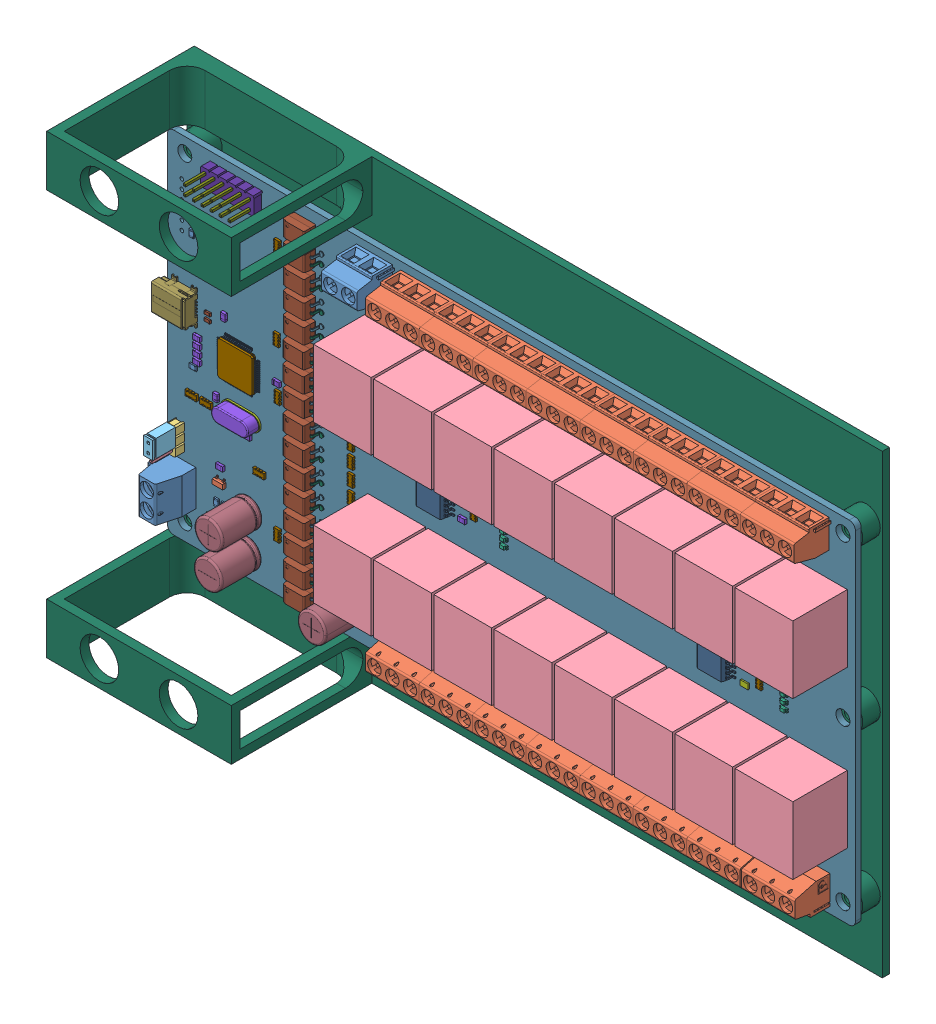
SolidWorks assembly Assem2, configuration Default. Lengths in mm. (continued)
Components (placement in the parent): (continued)
- 16_Channel_USB_Relay.step-1: 16_Channel_USB_Relay.step [Default] at (-11.9082 58.988 141.1455) size (200.04 103.47 20) (continued)
  - U12.step-1: U12.step [Default] at origin size (10 4.58 3.85) (continued)
    - User_Library-PC817_Gullwing.step-1: User_Library-PC817_Gullwing.step [Default] at (39.6975 47.1295 2.1) x (0 -1 0) z (-1 0 0) size (4.58 3.85 10) (continued)
      - User_Library-PC817_Gullwing_Gullwing_Pin_MIR_MIR.step-1: User_Library-PC817_Gullwing_Gullwing_Pin_MIR_MIR.step [Default] at (13.5652 -2.1015 0.2722) x (-1 0 0) z (0 0 -1) size (1.2 2.23 1.87)
  - U11.step-1: U11.step [Default] at origin size (10 4.58 3.85)
    - User_Library-PC817_Gullwing.step-1: User_Library-PC817_Gullwing.step [Default] at (39.6213 53.2509 2.1) x (0 -1 0) z (-1 0 0) size (4.58 3.85 10)
      - User_Library-PC817_Gullwing_PC817_Body.step-1: User_Library-PC817_Gullwing_PC817_Body.step [Default] at origin size (4.58 3.5 6.5)
      - User_Library-PC817_Gullwing_Gullwing_Pin.step-1: User_Library-PC817_Gullwing_Gullwing_Pin.step [Default] at (-13.5652 -2.1015 -0.2722) size (1.2 2.23 1.87)
      - User_Library-PC817_Gullwing_Gullwing_Pin_MIR.step-1: User_Library-PC817_Gullwing_Gullwing_Pin_MIR.step [Default] at (13.5652 -2.1015 -0.2722) x (-1 0 0) z (0 0 -1) size (1.2 2.23 1.87)
      - User_Library-PC817_Gullwing_Gullwing_Pin_MIR1.step-1: User_Library-PC817_Gullwing_Gullwing_Pin_MIR1.step [Default] at (-13.5652 -2.1015 0.2722) size (1.2 2.23 1.87)
      - User_Library-PC817_Gullwing_Gullwing_Pin_MIR_MIR.step-1: User_Library-PC817_Gullwing_Gullwing_Pin_MIR_MIR.step [Default] at (13.5652 -2.1015 0.2722) x (-1 0 0) z (0 0 -1) size (1.2 2.23 1.87)
  - U10.step-1: U10.step [Default] at origin size (10 4.58 3.85)
    - User_Library-PC817_Gullwing.step-1: User_Library-PC817_Gullwing.step [Default] at (39.6213 59.2199 2.1) x (0 -1 0) z (-1 0 0) size (4.58 3.85 10)
      - User_Library-PC817_Gullwing_PC817_Body.step-1: User_Library-PC817_Gullwing_PC817_Body.step [Default] at origin size (4.58 3.5 6.5)
      - User_Library-PC817_Gullwing_Gullwing_Pin.step-1: User_Library-PC817_Gullwing_Gullwing_Pin.step [Default] at (-13.5652 -2.1015 -0.2722) size (1.2 2.23 1.87)
      - User_Library-PC817_Gullwing_Gullwing_Pin_MIR.step-1: User_Library-PC817_Gullwing_Gullwing_Pin_MIR.step [Default] at (13.5652 -2.1015 -0.2722) x (-1 0 0) z (0 0 -1) size (1.2 2.23 1.87)
      - User_Library-PC817_Gullwing_Gullwing_Pin_MIR1.step-1: User_Library-PC817_Gullwing_Gullwing_Pin_MIR1.step [Default] at (-13.5652 -2.1015 0.2722) size (1.2 2.23 1.87)
      - User_Library-PC817_Gullwing_Gullwing_Pin_MIR_MIR.step-1: User_Library-PC817_Gullwing_Gullwing_Pin_MIR_MIR.step [Default] at (13.5652 -2.1015 0.2722) x (-1 0 0) z (0 0 -1) size (1.2 2.23 1.87)
  - U9.step-1: U9.step [Default] at origin size (10 4.58 3.85)
    - User_Library-PC817_Gullwing.step-1: User_Library-PC817_Gullwing.step [Default] at (39.6975 65.2651 2.1) x (0 -1 0) z (-1 0 0) size (4.58 3.85 10)
      - User_Library-PC817_Gullwing_PC817_Body.step-1: User_Library-PC817_Gullwing_PC817_Body.step [Default] at origin size (4.58 3.5 6.5)
      - User_Library-PC817_Gullwing_Gullwing_Pin.step-1: User_Library-PC817_Gullwing_Gullwing_Pin.step [Default] at (-13.5652 -2.1015 -0.2722) size (1.2 2.23 1.87)
      - User_Library-PC817_Gullwing_Gullwing_Pin_MIR.step-1: User_Library-PC817_Gullwing_Gullwing_Pin_MIR.step [Default] at (13.5652 -2.1015 -0.2722) x (-1 0 0) z (0 0 -1) size (1.2 2.23 1.87)
      - User_Library-PC817_Gullwing_Gullwing_Pin_MIR1.step-1: User_Library-PC817_Gullwing_Gullwing_Pin_MIR1.step [Default] at (-13.5652 -2.1015 0.2722) size (1.2 2.23 1.87)
      - User_Library-PC817_Gullwing_Gullwing_Pin_MIR_MIR.step-1: User_Library-PC817_Gullwing_Gullwing_Pin_MIR_MIR.step [Default] at (13.5652 -2.1015 0.2722) x (-1 0 0) z (0 0 -1) size (1.2 2.23 1.87)
  - U8.step-1: U8.step [Default] at origin size (10 4.58 3.85)
    - User_Library-PC817_Gullwing.step-1: User_Library-PC817_Gullwing.step [Default] at (39.7229 71.3865 2.1) x (0 -1 0) z (-1 0 0) size (4.58 3.85 10)
      - User_Library-PC817_Gullwing_PC817_Body.step-1: User_Library-PC817_Gullwing_PC817_Body.step [Default] at origin size (4.58 3.5 6.5)
      - User_Library-PC817_Gullwing_Gullwing_Pin.step-1: User_Library-PC817_Gullwing_Gullwing_Pin.step [Default] at (-13.5652 -2.1015 -0.2722) size (1.2 2.23 1.87)
      - User_Library-PC817_Gullwing_Gullwing_Pin_MIR.step-1: User_Library-PC817_Gullwing_Gullwing_Pin_MIR.step [Default] at (13.5652 -2.1015 -0.2722) x (-1 0 0) z (0 0 -1) size (1.2 2.23 1.87)
      - User_Library-PC817_Gullwing_Gullwing_Pin_MIR1.step-1: User_Library-PC817_Gullwing_Gullwing_Pin_MIR1.step [Default] at (-13.5652 -2.1015 0.2722) size (1.2 2.23 1.87)
      - User_Library-PC817_Gullwing_Gullwing_Pin_MIR_MIR.step-1: User_Library-PC817_Gullwing_Gullwing_Pin_MIR_MIR.step [Default] at (13.5652 -2.1015 0.2722) x (-1 0 0) z (0 0 -1) size (1.2 2.23 1.87)
  - U7.step-1: U7.step [Default] at origin size (10 4.58 3.85)
    - User_Library-PC817_Gullwing.step-1: User_Library-PC817_Gullwing.step [Default] at (39.7737 77.4317 2.1) x (0 -1 0) z (-1 0 0) size (4.58 3.85 10)
      - User_Library-PC817_Gullwing_PC817_Body.step-1: User_Library-PC817_Gullwing_PC817_Body.step [Default] at origin size (4.58 3.5 6.5)
      - User_Library-PC817_Gullwing_Gullwing_Pin.step-1: User_Library-PC817_Gullwing_Gullwing_Pin.step [Default] at (-13.5652 -2.1015 -0.2722) size (1.2 2.23 1.87)
      - User_Library-PC817_Gullwing_Gullwing_Pin_MIR.step-1: User_Library-PC817_Gullwing_Gullwing_Pin_MIR.step [Default] at (13.5652 -2.1015 -0.2722) x (-1 0 0) z (0 0 -1) size (1.2 2.23 1.87)
      - User_Library-PC817_Gullwing_Gullwing_Pin_MIR1.step-1: User_Library-PC817_Gullwing_Gullwing_Pin_MIR1.step [Default] at (-13.5652 -2.1015 0.2722) size (1.2 2.23 1.87)
      - User_Library-PC817_Gullwing_Gullwing_Pin_MIR_MIR.step-1: User_Library-PC817_Gullwing_Gullwing_Pin_MIR_MIR.step [Default] at (13.5652 -2.1015 0.2722) x (-1 0 0) z (0 0 -1) size (1.2 2.23 1.87)
  - U6.step-1: U6.step [Default] at origin size (10 4.58 3.85)
    - User_Library-PC817_Gullwing.step-1: User_Library-PC817_Gullwing.step [Default] at (39.7737 83.2991 2.1) x (0 -1 0) z (-1 0 0) size (4.58 3.85 10)
      - User_Library-PC817_Gullwing_PC817_Body.step-1: User_Library-PC817_Gullwing_PC817_Body.step [Default] at origin size (4.58 3.5 6.5)
      - User_Library-PC817_Gullwing_Gullwing_Pin.step-1: User_Library-PC817_Gullwing_Gullwing_Pin.step [Default] at (-13.5652 -2.1015 -0.2722) size (1.2 2.23 1.87)
      - User_Library-PC817_Gullwing_Gullwing_Pin_MIR.step-1: User_Library-PC817_Gullwing_Gullwing_Pin_MIR.step [Default] at (13.5652 -2.1015 -0.2722) x (-1 0 0) z (0 0 -1) size (1.2 2.23 1.87)
      - User_Library-PC817_Gullwing_Gullwing_Pin_MIR1.step-1: User_Library-PC817_Gullwing_Gullwing_Pin_MIR1.step [Default] at (-13.5652 -2.1015 0.2722) size (1.2 2.23 1.87)
      - User_Library-PC817_Gullwing_Gullwing_Pin_MIR_MIR.step-1: User_Library-PC817_Gullwing_Gullwing_Pin_MIR_MIR.step [Default] at (13.5652 -2.1015 0.2722) x (-1 0 0) z (0 0 -1) size (1.2 2.23 1.87)
  - U5.step-1: U5.step [Default] at origin size (10 4.58 3.85)
    - User_Library-PC817_Gullwing.step-1: User_Library-PC817_Gullwing.step [Default] at (39.7737 89.2681 2.1) x (0 -1 0) z (-1 0 0) size (4.58 3.85 10)
      - User_Library-PC817_Gullwing_PC817_Body.step-1: User_Library-PC817_Gullwing_PC817_Body.step [Default] at origin size (4.58 3.5 6.5)
      - User_Library-PC817_Gullwing_Gullwing_Pin.step-1: User_Library-PC817_Gullwing_Gullwing_Pin.step [Default] at (-13.5652 -2.1015 -0.2722) size (1.2 2.23 1.87)
      - User_Library-PC817_Gullwing_Gullwing_Pin_MIR.step-1: User_Library-PC817_Gullwing_Gullwing_Pin_MIR.step [Default] at (13.5652 -2.1015 -0.2722) x (-1 0 0) z (0 0 -1) size (1.2 2.23 1.87)
      - User_Library-PC817_Gullwing_Gullwing_Pin_MIR1.step-1: User_Library-PC817_Gullwing_Gullwing_Pin_MIR1.step [Default] at (-13.5652 -2.1015 0.2722) size (1.2 2.23 1.87)
      - User_Library-PC817_Gullwing_Gullwing_Pin_MIR_MIR.step-1: User_Library-PC817_Gullwing_Gullwing_Pin_MIR_MIR.step [Default] at (13.5652 -2.1015 0.2722) x (-1 0 0) z (0 0 -1) size (1.2 2.23 1.87)
  - U4.step-1: U4.step [Default] at origin size (10 4.58 3.85)
    - User_Library-PC817_Gullwing.step-1: User_Library-PC817_Gullwing.step [Default] at (39.7737 95.1355 2.1) x (0 -1 0) z (-1 0 0) size (4.58 3.85 10)
      - User_Library-PC817_Gullwing_PC817_Body.step-1: User_Library-PC817_Gullwing_PC817_Body.step [Default] at origin size (4.58 3.5 6.5)
      - User_Library-PC817_Gullwing_Gullwing_Pin.step-1: User_Library-PC817_Gullwing_Gullwing_Pin.step [Default] at (-13.5652 -2.1015 -0.2722) size (1.2 2.23 1.87)
      - User_Library-PC817_Gullwing_Gullwing_Pin_MIR.step-1: User_Library-PC817_Gullwing_Gullwing_Pin_MIR.step [Default] at (13.5652 -2.1015 -0.2722) x (-1 0 0) z (0 0 -1) size (1.2 2.23 1.87)
      - User_Library-PC817_Gullwing_Gullwing_Pin_MIR1.step-1: User_Library-PC817_Gullwing_Gullwing_Pin_MIR1.step [Default] at (-13.5652 -2.1015 0.2722) size (1.2 2.23 1.87)
      - User_Library-PC817_Gullwing_Gullwing_Pin_MIR_MIR.step-1: User_Library-PC817_Gullwing_Gullwing_Pin_MIR_MIR.step [Default] at (13.5652 -2.1015 0.2722) x (-1 0 0) z (0 0 -1) size (1.2 2.23 1.87)
  - P1.step-1: P1.step [Default] at origin size (15.24 5.08 11.54)
    - STEP-61301221121-rev1.step-1: STEP-61301221121-rev1.step [Default] at (19.7712 96.3422 1.3) x (-1 0 0) z (0 1 0) size (15.24 11.54 5.08)
      - 6130xx21121_PIN.step-1: 6130xx21121_PIN.step [Default] at (-6.35 1.5 0) x (1 0 0) z (0 -1 0) size (0.64 0.64 11.54)
      - 6130xx21121_PIN.step-2: 6130xx21121_PIN.step [Default] at (-6.35 1.5 -2.54) x (1 0 0) z (0 -1 0) size (0.64 0.64 11.54)
      - 6130xx21121_PIN.step-3: 6130xx21121_PIN.step [Default] at (-3.81 1.5 0) x (1 0 0) z (0 -1 0) size (0.64 0.64 11.54)
      - 6130xx21121_PIN.step-4: 6130xx21121_PIN.step [Default] at (-3.81 1.5 -2.54) x (1 0 0) z (0 -1 0) size (0.64 0.64 11.54)
      - 6130xx21121_PIN.step-5: 6130xx21121_PIN.step [Default] at (-1.27 1.5 0) x (1 0 0) z (0 -1 0) size (0.64 0.64 11.54)
      - 6130xx21121_PIN.step-6: 6130xx21121_PIN.step [Default] at (-1.27 1.5 -2.54) x (1 0 0) z (0 -1 0) size (0.64 0.64 11.54)
      - 6130xx21121_PIN.step-7: 6130xx21121_PIN.step [Default] at (1.27 1.5 0) x (1 0 0) z (0 -1 0) size (0.64 0.64 11.54)
      - 6130xx21121_PIN.step-8: 6130xx21121_PIN.step [Default] at (1.27 1.5 -2.54) x (1 0 0) z (0 -1 0) size (0.64 0.64 11.54)
      - 6130xx21121_PIN.step-9: 6130xx21121_PIN.step [Default] at (3.81 1.5 0) x (1 0 0) z (0 -1 0) size (0.64 0.64 11.54)
      - 6130xx21121_PIN.step-10: 6130xx21121_PIN.step [Default] at (3.81 1.5 -2.54) x (1 0 0) z (0 -1 0) size (0.64 0.64 11.54)
      - 6130xx21121_PIN.step-11: 6130xx21121_PIN.step [Default] at (6.35 1.5 0) x (1 0 0) z (0 -1 0) size (0.64 0.64 11.54)
      - 6130xx21121_PIN.step-12: 6130xx21121_PIN.step [Default] at (6.35 1.5 -2.54) x (1 0 0) z (0 -1 0) size (0.64 0.64 11.54)
      - 61301221121.step-1: 61301221121.step [Default] at origin size (15.24 2.54 5.08)
  - P5.step-1: P5.step [Default] at origin size (8.1 10.73 13.5)
    - 1729128_07.step-1: 1729128_07.step [Default] at (0.7762 20.5414 0) x (-1 0 0) z (0 1 0) size (8.1 13.5 10.73)
      - mkdsn_1.5-2-5.08.step-1: mkdsn_1.5-2-5.08.step [Default] at (-39.331 -15.5089 -8.19) x (-1 0 0) z (0 0 -1) size (8.1 13.5 10.73)
  - U2.step-1: U2.step [Default] at origin size (8.15 10.72 7.75)
    - SOT-223.step-1: SOT-223.step [Default] at (14.0941 7.1499 0) x (-1 0 0) z (0 0 1) size (8.15 10.72 7.75)
  - R13.step-1: R13.step [Default] at origin size (1.6 3.2 0.65)
    - User_Library-resnet.step-1: User_Library-resnet.step [Default] at (31.7979 15.3035 0) x (0 1 0) z (1 0 0) size (3.2 0.65 1.6)
  - R3.step-1: R3.step [Default] at origin size (1.25 2 0.47)
    - SW3dPS-R0805.step-1: SW3dPS-R0805.step [Default] at (16.4057 14.5159 -0.05) x (0 -1 0) z (0 0 1) size (2 1.25 0.47)
  - R4.step-1: R4.step [Default] at origin size (1.25 2 0.47)
    - SW3dPS-R0805.step-1: SW3dPS-R0805.step [Default] at (14.3991 14.5159 -0.05) x (0 -1 0) z (0 0 1) size (2 1.25 0.47)
  - D1.step-1: D1.step [Default] at origin size (3 2.5 1.1)
    - CircuitWorks-SOT-23.step-1: CircuitWorks-SOT-23.step [Default] at (15.4911 19.9515 0.5541) x (1 0 0) z (0 -1 0) size (3 1.1 2.5)
  - C12.step-1: C12.step [Default] at origin size (2 1.31 0.76)
    - SW3DPS-CAPACITOR_0805-DEFAULT.step-1: SW3DPS-CAPACITOR_0805-DEFAULT.step [Default] at (15.5419 23.9139 0) x (1 0 0) z (0 -1 0) size (2 0.76 1.31)
  - K1.step-1: K1.step [Default] at origin size (2.61 7.64 12.07)
    - jmper.step-1: jmper.step [Default] at (3.7564 25.7682 1.25) x (-0.008727 0.999962 0) z (0.999962 0.008727 0) size (7.62 11.54 2.54)
      - 61300311121.step-1: 61300311121.step [Default] at origin size (7.62 2.54 2.54)
      - 6130xx11121_PIN.step-1: 6130xx11121_PIN.step [Default] at (-2.54 1.5 0) x (1 0 0) z (0 -1 0) size (0.64 0.64 11.54)
      - 6130xx11121_PIN.step-2: 6130xx11121_PIN.step [Default] at (0 1.5 0) x (1 0 0) z (0 -1 0) size (0.64 0.64 11.54)
      - 6130xx11121_PIN.step-3: 6130xx11121_PIN.step [Default] at (2.54 1.5 0) x (1 0 0) z (0 -1 0) size (0.64 0.64 11.54)
    - pcb_connector_999-19-210-00.step-1: pcb_connector_999-19-210-00.step [Default] at (3.7563 27.0383 2.55) x (0 -1 0) z (-1 0 0) size (5 6.5 2.54)
  - R1.step-1: R1.step [Default] at origin size (3.2 1.6 0.65)
    - User_Library-resnet.step-1: User_Library-resnet.step [Default] at (26.6925 27.9525 0) x (-1 0 0) z (0 1 0) size (3.2 0.65 1.6)
  - C2.step-1: C2.step [Default] at origin size (2 1.31 0.76)
    - SW3DPS-CAPACITOR_0805-DEFAULT.step-1: SW3DPS-CAPACITOR_0805-DEFAULT.step [Default] at (23.3143 35.3947 0) x (1 0 0) z (0 -1 0) size (2 0.76 1.31)
  - C1.step-1: C1.step [Default] at origin size (2 1.31 0.76)
    - SW3DPS-CAPACITOR_0805-DEFAULT.step-1: SW3DPS-CAPACITOR_0805-DEFAULT.step [Default] at (19.7583 35.3947 0) x (1 0 0) z (0 -1 0) size (2 0.76 1.31)
  - X1.step-1: X1.step [Default] at origin size (10.98 4.49 6.6)
    - User_Library-HC49S-1.step-1: User_Library-HC49S-1.step [Default] at (23.8241 39.3469 0) x (-1 0 0) z (0 0 1) size (10.98 4.49 6.6)
      - User_Library-HC49S-1_Fusion.step-1: User_Library-HC49S-1_Fusion.step [Default] at origin size (5.32 0.44 3)
      - User_Library-HC49S-1_Fillet.step-1: User_Library-HC49S-1_Fillet.step [Default] at origin size (10.98 4.49 0.5)
      - User_Library-HC49S-1_Fillet002.step-1: User_Library-HC49S-1_Fillet002.step [Default] at origin size (10.48 3.99 3.5)
  - R7.step-1: R7.step [Default] at origin size (3.2 1.6 0.65)
    - User_Library-resnet.step-1: User_Library-resnet.step [Default] at (11.4957 37.6049 0) x (1 0 0) z (0 -1 0) size (3.2 0.65 1.6)
  - R6.step-1: R6.step [Default] at origin size (3.2 1.6 0.65)
    - User_Library-resnet.step-1: User_Library-resnet.step [Default] at (7.4317 37.5795 0) x (1 0 0) z (0 -1 0) size (3.2 0.65 1.6)
  - C7.step-1: C7.step [Default] at origin size (1.31 2 0.76)
    - SW3DPS-CAPACITOR_0805-DEFAULT.step-1: SW3DPS-CAPACITOR_0805-DEFAULT.step [Default] at (14.3735 40.5765 0) x (0 -1 0) z (-1 0 0) size (2 0.76 1.31)
  - R9.step-1: R9.step [Default] at origin size (2 1.25 0.47)
    - SW3dPS-R0805.step-1: SW3dPS-R0805.step [Default] at (7.7695 44.6149 -0.05) x (-1 0 0) z (0 0 1) size (2 1.25 0.47)
  - C4.step-1: C4.step [Default] at origin size (2 1.31 0.76)
    - SW3DPS-CAPACITOR_0805-DEFAULT.step-1: SW3DPS-CAPACITOR_0805-DEFAULT.step [Default] at (8.9889 46.5709 0) x (-1 0 0) z (0 1 0) size (2 0.76 1.31)
  - C8.step-1: C8.step [Default] at origin size (2 1.31 0.76)
    - SW3DPS-CAPACITOR_0805-DEFAULT.step-1: SW3DPS-CAPACITOR_0805-DEFAULT.step [Default] at (8.9889 48.5267 0) x (-1 0 0) z (0 1 0) size (2 0.76 1.31)
  - C10.step-1: C10.step [Default] at origin size (2 1.31 0.76)
    - SW3DPS-CAPACITOR_0805-DEFAULT.step-1: SW3DPS-CAPACITOR_0805-DEFAULT.step [Default] at (8.9889 50.5333 0) x (-1 0 0) z (0 1 0) size (2 0.76 1.31)
  - C6.step-1: C6.step [Default] at origin size (2 1.31 0.76)
    - SW3DPS-CAPACITOR_0805-DEFAULT.step-1: SW3DPS-CAPACITOR_0805-DEFAULT.step [Default] at (8.9889 52.5145 0) x (-1 0 0) z (0 1 0) size (2 0.76 1.31)
  - R12.step-1: R12.step [Default] at origin size (1.6 3.2 0.65)
    - User_Library-resnet.step-1: User_Library-resnet.step [Default] at (31.8995 49.2633 0) x (0 1 0) z (1 0 0) size (3.2 0.65 1.6)
  - C9.step-1: C9.step [Default] at origin size (2 1.31 0.76)
    - SW3DPS-CAPACITOR_0805-DEFAULT.step-1: SW3DPS-CAPACITOR_0805-DEFAULT.step [Default] at (31.6709 52.6921 0) x (1 0 0) z (0 -1 0) size (2 0.76 1.31)
  - U3.step-1: U3.step [Default] at origin size (12 12 1.2)
    - User_Library-TQFP64_Grid_0_5.step-1: User_Library-TQFP64_Grid_0_5.step [Default] at (20.5457 51.4475 0) x (-1 0 0) z (0 1 0) size (12 1.2 12)
      - User_Library-TQFP64_Grid_0.5_TQFP64_Koerper_2.step-1: User_Library-TQFP64_Grid_0.5_TQFP64_Koerper_2.step [Default] at origin size (10 1.05 10)
      - User_Library-TQFP64_Grid_0.5_TQFP_PIN_2.step-1: User_Library-TQFP64_Grid_0.5_TQFP_PIN_2.step [Default] at (-3.75 0 6) size (0.27 0.77 1.5)
      - User_Library-TQFP64_Grid_0.5_TQFP_PIN_2.step-2: User_Library-TQFP64_Grid_0.5_TQFP_PIN_2.step [Default] at (-3.25 0 6) size (0.27 0.77 1.5)
      - User_Library-TQFP64_Grid_0.5_TQFP_PIN_2.step-3: User_Library-TQFP64_Grid_0.5_TQFP_PIN_2.step [Default] at (-2.75 0 6) size (0.27 0.77 1.5)
      - User_Library-TQFP64_Grid_0.5_TQFP_PIN_2.step-4: User_Library-TQFP64_Grid_0.5_TQFP_PIN_2.step [Default] at (-2.25 0 6) size (0.27 0.77 1.5)
      - User_Library-TQFP64_Grid_0.5_TQFP_PIN_2.step-5: User_Library-TQFP64_Grid_0.5_TQFP_PIN_2.step [Default] at (-1.75 0 6) size (0.27 0.77 1.5)
      - User_Library-TQFP64_Grid_0.5_TQFP_PIN_2.step-6: User_Library-TQFP64_Grid_0.5_TQFP_PIN_2.step [Default] at (-1.25 0 6) size (0.27 0.77 1.5)
      - User_Library-TQFP64_Grid_0.5_TQFP_PIN_2.step-7: User_Library-TQFP64_Grid_0.5_TQFP_PIN_2.step [Default] at (-0.75 0 6) size (0.27 0.77 1.5)
      - User_Library-TQFP64_Grid_0.5_TQFP_PIN_2.step-8: User_Library-TQFP64_Grid_0.5_TQFP_PIN_2.step [Default] at (-0.25 0 6) size (0.27 0.77 1.5)
      - User_Library-TQFP64_Grid_0.5_TQFP_PIN_2.step-9: User_Library-TQFP64_Grid_0.5_TQFP_PIN_2.step [Default] at (0.25 0 6) size (0.27 0.77 1.5)
      - User_Library-TQFP64_Grid_0.5_TQFP_PIN_2.step-10: User_Library-TQFP64_Grid_0.5_TQFP_PIN_2.step [Default] at (0.75 0 6) size (0.27 0.77 1.5)
      - User_Library-TQFP64_Grid_0.5_TQFP_PIN_2.step-11: User_Library-TQFP64_Grid_0.5_TQFP_PIN_2.step [Default] at (1.25 0 6) size (0.27 0.77 1.5)
      - User_Library-TQFP64_Grid_0.5_TQFP_PIN_2.step-12: User_Library-TQFP64_Grid_0.5_TQFP_PIN_2.step [Default] at (1.75 0 6) size (0.27 0.77 1.5)
      - User_Library-TQFP64_Grid_0.5_TQFP_PIN_2.step-13: User_Library-TQFP64_Grid_0.5_TQFP_PIN_2.step [Default] at (2.25 0 6) size (0.27 0.77 1.5)
      - User_Library-TQFP64_Grid_0.5_TQFP_PIN_2.step-14: User_Library-TQFP64_Grid_0.5_TQFP_PIN_2.step [Default] at (2.75 0 6) size (0.27 0.77 1.5)
      - User_Library-TQFP64_Grid_0.5_TQFP_PIN_2.step-15: User_Library-TQFP64_Grid_0.5_TQFP_PIN_2.step [Default] at (3.25 0 6) size (0.27 0.77 1.5)
      - User_Library-TQFP64_Grid_0.5_TQFP_PIN_2.step-16: User_Library-TQFP64_Grid_0.5_TQFP_PIN_2.step [Default] at (3.75 0 6) size (0.27 0.77 1.5)
      - User_Library-TQFP64_Grid_0.5_TQFP_PIN_2.step-17: User_Library-TQFP64_Grid_0.5_TQFP_PIN_2.step [Default] at (6 0 3.75) x (0 0 -1) z (1 0 0) size (0.27 0.77 1.5)
      - User_Library-TQFP64_Grid_0.5_TQFP_PIN_2.step-18: User_Library-TQFP64_Grid_0.5_TQFP_PIN_2.step [Default] at (6 0 3.25) x (0 0 -1) z (1 0 0) size (0.27 0.77 1.5)
      - User_Library-TQFP64_Grid_0.5_TQFP_PIN_2.step-19: User_Library-TQFP64_Grid_0.5_TQFP_PIN_2.step [Default] at (6 0 2.75) x (0 0 -1) z (1 0 0) size (0.27 0.77 1.5)
      - User_Library-TQFP64_Grid_0.5_TQFP_PIN_2.step-20: User_Library-TQFP64_Grid_0.5_TQFP_PIN_2.step [Default] at (6 0 2.25) x (0 0 -1) z (1 0 0) size (0.27 0.77 1.5)
      - User_Library-TQFP64_Grid_0.5_TQFP_PIN_2.step-21: User_Library-TQFP64_Grid_0.5_TQFP_PIN_2.step [Default] at (6 0 1.75) x (0 0 -1) z (1 0 0) size (0.27 0.77 1.5)
      - User_Library-TQFP64_Grid_0.5_TQFP_PIN_2.step-22: User_Library-TQFP64_Grid_0.5_TQFP_PIN_2.step [Default] at (6 0 1.25) x (0 0 -1) z (1 0 0) size (0.27 0.77 1.5)
      - User_Library-TQFP64_Grid_0.5_TQFP_PIN_2.step-23: User_Library-TQFP64_Grid_0.5_TQFP_PIN_2.step [Default] at (6 0 0.75) x (0 0 -1) z (1 0 0) size (0.27 0.77 1.5)
      - User_Library-TQFP64_Grid_0.5_TQFP_PIN_2.step-24: User_Library-TQFP64_Grid_0.5_TQFP_PIN_2.step [Default] at (6 0 0.25) x (0 0 -1) z (1 0 0) size (0.27 0.77 1.5)
      - User_Library-TQFP64_Grid_0.5_TQFP_PIN_2.step-25: User_Library-TQFP64_Grid_0.5_TQFP_PIN_2.step [Default] at (6 0 -0.25) x (0 0 -1) z (1 0 0) size (0.27 0.77 1.5)
      - User_Library-TQFP64_Grid_0.5_TQFP_PIN_2.step-26: User_Library-TQFP64_Grid_0.5_TQFP_PIN_2.step [Default] at (6 0 -0.75) x (0 0 -1) z (1 0 0) size (0.27 0.77 1.5)
      - User_Library-TQFP64_Grid_0.5_TQFP_PIN_2.step-27: User_Library-TQFP64_Grid_0.5_TQFP_PIN_2.step [Default] at (6 0 -1.25) x (0 0 -1) z (1 0 0) size (0.27 0.77 1.5)
      - User_Library-TQFP64_Grid_0.5_TQFP_PIN_2.step-28: User_Library-TQFP64_Grid_0.5_TQFP_PIN_2.step [Default] at (6 0 -1.75) x (0 0 -1) z (1 0 0) size (0.27 0.77 1.5)
      - User_Library-TQFP64_Grid_0.5_TQFP_PIN_2.step-29: User_Library-TQFP64_Grid_0.5_TQFP_PIN_2.step [Default] at (6 0 -2.25) x (0 0 -1) z (1 0 0) size (0.27 0.77 1.5)
      - User_Library-TQFP64_Grid_0.5_TQFP_PIN_2.step-30: User_Library-TQFP64_Grid_0.5_TQFP_PIN_2.step [Default] at (6 0 -2.75) x (0 0 -1) z (1 0 0) size (0.27 0.77 1.5)
      - User_Library-TQFP64_Grid_0.5_TQFP_PIN_2.step-31: User_Library-TQFP64_Grid_0.5_TQFP_PIN_2.step [Default] at (6 0 -3.25) x (0 0 -1) z (1 0 0) size (0.27 0.77 1.5)
      - User_Library-TQFP64_Grid_0.5_TQFP_PIN_2.step-32: User_Library-TQFP64_Grid_0.5_TQFP_PIN_2.step [Default] at (6 0 -3.75) x (0 0 -1) z (1 0 0) size (0.27 0.77 1.5)
      - User_Library-TQFP64_Grid_0.5_TQFP_PIN_2.step-33: User_Library-TQFP64_Grid_0.5_TQFP_PIN_2.step [Default] at (3.75 0 -6) x (-1 0 0) z (0 0 -1) size (0.27 0.77 1.5)
      - User_Library-TQFP64_Grid_0.5_TQFP_PIN_2.step-34: User_Library-TQFP64_Grid_0.5_TQFP_PIN_2.step [Default] at (3.25 0 -6) x (-1 0 0) z (0 0 -1) size (0.27 0.77 1.5)
      - User_Library-TQFP64_Grid_0.5_TQFP_PIN_2.step-35: User_Library-TQFP64_Grid_0.5_TQFP_PIN_2.step [Default] at (2.75 0 -6) x (-1 0 0) z (0 0 -1) size (0.27 0.77 1.5)
      - User_Library-TQFP64_Grid_0.5_TQFP_PIN_2.step-36: User_Library-TQFP64_Grid_0.5_TQFP_PIN_2.step [Default] at (2.25 0 -6) x (-1 0 0) z (0 0 -1) size (0.27 0.77 1.5)
      - User_Library-TQFP64_Grid_0.5_TQFP_PIN_2.step-37: User_Library-TQFP64_Grid_0.5_TQFP_PIN_2.step [Default] at (1.75 0 -6) x (-1 0 0) z (0 0 -1) size (0.27 0.77 1.5)
      - User_Library-TQFP64_Grid_0.5_TQFP_PIN_2.step-38: User_Library-TQFP64_Grid_0.5_TQFP_PIN_2.step [Default] at (1.25 0 -6) x (-1 0 0) z (0 0 -1) size (0.27 0.77 1.5)
      - User_Library-TQFP64_Grid_0.5_TQFP_PIN_2.step-39: User_Library-TQFP64_Grid_0.5_TQFP_PIN_2.step [Default] at (0.75 0 -6) x (-1 0 0) z (0 0 -1) size (0.27 0.77 1.5)
      - User_Library-TQFP64_Grid_0.5_TQFP_PIN_2.step-40: User_Library-TQFP64_Grid_0.5_TQFP_PIN_2.step [Default] at (0.25 0 -6) x (-1 0 0) z (0 0 -1) size (0.27 0.77 1.5)
      - User_Library-TQFP64_Grid_0.5_TQFP_PIN_2.step-41: User_Library-TQFP64_Grid_0.5_TQFP_PIN_2.step [Default] at (-0.25 0 -6) x (-1 0 0) z (0 0 -1) size (0.27 0.77 1.5)
      - User_Library-TQFP64_Grid_0.5_TQFP_PIN_2.step-42: User_Library-TQFP64_Grid_0.5_TQFP_PIN_2.step [Default] at (-0.75 0 -6) x (-1 0 0) z (0 0 -1) size (0.27 0.77 1.5)
      - User_Library-TQFP64_Grid_0.5_TQFP_PIN_2.step-43: User_Library-TQFP64_Grid_0.5_TQFP_PIN_2.step [Default] at (-1.25 0 -6) x (-1 0 0) z (0 0 -1) size (0.27 0.77 1.5)
      - User_Library-TQFP64_Grid_0.5_TQFP_PIN_2.step-44: User_Library-TQFP64_Grid_0.5_TQFP_PIN_2.step [Default] at (-1.75 0 -6) x (-1 0 0) z (0 0 -1) size (0.27 0.77 1.5)
      - User_Library-TQFP64_Grid_0.5_TQFP_PIN_2.step-45: User_Library-TQFP64_Grid_0.5_TQFP_PIN_2.step [Default] at (-2.25 0 -6) x (-1 0 0) z (0 0 -1) size (0.27 0.77 1.5)
      - User_Library-TQFP64_Grid_0.5_TQFP_PIN_2.step-46: User_Library-TQFP64_Grid_0.5_TQFP_PIN_2.step [Default] at (-2.75 0 -6) x (-1 0 0) z (0 0 -1) size (0.27 0.77 1.5)
      - User_Library-TQFP64_Grid_0.5_TQFP_PIN_2.step-47: User_Library-TQFP64_Grid_0.5_TQFP_PIN_2.step [Default] at (-3.25 0 -6) x (-1 0 0) z (0 0 -1) size (0.27 0.77 1.5)
      - User_Library-TQFP64_Grid_0.5_TQFP_PIN_2.step-48: User_Library-TQFP64_Grid_0.5_TQFP_PIN_2.step [Default] at (-3.75 0 -6) x (-1 0 0) z (0 0 -1) size (0.27 0.77 1.5)
      - User_Library-TQFP64_Grid_0.5_TQFP_PIN_2.step-49: User_Library-TQFP64_Grid_0.5_TQFP_PIN_2.step [Default] at (-6 0 -3.75) x (0 0 1) z (-1 0 0) size (0.27 0.77 1.5)
      - User_Library-TQFP64_Grid_0.5_TQFP_PIN_2.step-50: User_Library-TQFP64_Grid_0.5_TQFP_PIN_2.step [Default] at (-6 0 -3.25) x (0 0 1) z (-1 0 0) size (0.27 0.77 1.5)
      - User_Library-TQFP64_Grid_0.5_TQFP_PIN_2.step-51: User_Library-TQFP64_Grid_0.5_TQFP_PIN_2.step [Default] at (-6 0 -2.75) x (0 0 1) z (-1 0 0) size (0.27 0.77 1.5)
      - User_Library-TQFP64_Grid_0.5_TQFP_PIN_2.step-52: User_Library-TQFP64_Grid_0.5_TQFP_PIN_2.step [Default] at (-6 0 -2.25) x (0 0 1) z (-1 0 0) size (0.27 0.77 1.5)
      - User_Library-TQFP64_Grid_0.5_TQFP_PIN_2.step-53: User_Library-TQFP64_Grid_0.5_TQFP_PIN_2.step [Default] at (-6 0 -1.75) x (0 0 1) z (-1 0 0) size (0.27 0.77 1.5)
      - User_Library-TQFP64_Grid_0.5_TQFP_PIN_2.step-54: User_Library-TQFP64_Grid_0.5_TQFP_PIN_2.step [Default] at (-6 0 -1.25) x (0 0 1) z (-1 0 0) size (0.27 0.77 1.5)
      - User_Library-TQFP64_Grid_0.5_TQFP_PIN_2.step-55: User_Library-TQFP64_Grid_0.5_TQFP_PIN_2.step [Default] at (-6 0 -0.75) x (0 0 1) z (-1 0 0) size (0.27 0.77 1.5)
      - User_Library-TQFP64_Grid_0.5_TQFP_PIN_2.step-56: User_Library-TQFP64_Grid_0.5_TQFP_PIN_2.step [Default] at (-6 0 -0.25) x (0 0 1) z (-1 0 0) size (0.27 0.77 1.5)
      - User_Library-TQFP64_Grid_0.5_TQFP_PIN_2.step-57: User_Library-TQFP64_Grid_0.5_TQFP_PIN_2.step [Default] at (-6 0 0.25) x (0 0 1) z (-1 0 0) size (0.27 0.77 1.5)
      - User_Library-TQFP64_Grid_0.5_TQFP_PIN_2.step-58: User_Library-TQFP64_Grid_0.5_TQFP_PIN_2.step [Default] at (-6 0 0.75) x (0 0 1) z (-1 0 0) size (0.27 0.77 1.5)
      - User_Library-TQFP64_Grid_0.5_TQFP_PIN_2.step-59: User_Library-TQFP64_Grid_0.5_TQFP_PIN_2.step [Default] at (-6 0 1.25) x (0 0 1) z (-1 0 0) size (0.27 0.77 1.5)
      - User_Library-TQFP64_Grid_0.5_TQFP_PIN_2.step-60: User_Library-TQFP64_Grid_0.5_TQFP_PIN_2.step [Default] at (-6 0 1.75) x (0 0 1) z (-1 0 0) size (0.27 0.77 1.5)
      - User_Library-TQFP64_Grid_0.5_TQFP_PIN_2.step-61: User_Library-TQFP64_Grid_0.5_TQFP_PIN_2.step [Default] at (-6 0 2.25) x (0 0 1) z (-1 0 0) size (0.27 0.77 1.5)
      - User_Library-TQFP64_Grid_0.5_TQFP_PIN_2.step-62: User_Library-TQFP64_Grid_0.5_TQFP_PIN_2.step [Default] at (-6 0 2.75) x (0 0 1) z (-1 0 0) size (0.27 0.77 1.5)
      - User_Library-TQFP64_Grid_0.5_TQFP_PIN_2.step-63: User_Library-TQFP64_Grid_0.5_TQFP_PIN_2.step [Default] at (-6 0 3.25) x (0 0 1) z (-1 0 0) size (0.27 0.77 1.5)
      - User_Library-TQFP64_Grid_0.5_TQFP_PIN_2.step-64: User_Library-TQFP64_Grid_0.5_TQFP_PIN_2.step [Default] at (-6 0 3.75) x (0 0 1) z (-1 0 0) size (0.27 0.77 1.5)
  - R11.step-1: R11.step [Default] at origin size (1.6 3.2 0.65)
    - User_Library-resnet.step-1: User_Library-resnet.step [Default] at (31.6201 63.3857 0) x (0 1 0) z (1 0 0) size (3.2 0.65 1.6)
  - C5.step-1: C5.step [Default] at origin size (1.31 2 0.76)
    - SW3DPS-CAPACITOR_0805-DEFAULT.step-1: SW3DPS-CAPACITOR_0805-DEFAULT.step [Default] at (16.6089 61.5313 0) x (0 1 0) z (1 0 0) size (2 0.76 1.31)
  - VR1.step-1: VR1.step [Default] at origin size (1.6 0.86 0.51)
    - SW3DPS-RESISTOR_0603-DEFAULT.step-1: SW3DPS-RESISTOR_0603-DEFAULT.step [Default] at (11.8845 58.1279 0) x (1 0 0) z (0 -1 0) size (1.6 0.51 0.86)
  - VR2.step-1: VR2.step [Default] at origin size (1.6 0.86 0.51)
    - SW3DPS-RESISTOR_0603-DEFAULT.step-1: SW3DPS-RESISTOR_0603-DEFAULT.step [Default] at (11.8845 59.8805 0) x (1 0 0) z (0 -1 0) size (1.6 0.51 0.86)
  - J2.step-1: J2.step [Default] at origin size (9.25 9.9 4.93)
    - usb_a-usb_b-m5-smd-c.step-1: usb_a-usb_b-m5-smd-c.step [Default] at (-0.5153 59.5249 0) x (0 -1 0) z (-1 0 0) size (9.9 4.93 9.25)
  - R5.step-1: R5.step [Default] at origin size (3.2 1.6 0.65)
    - User_Library-resnet.step-1: User_Library-resnet.step [Default] at (18.4375 72.1739 0) x (-1 0 0) z (0 1 0) size (3.2 0.65 1.6)
  - R2.step-1: R2.step [Default] at origin size (3.2 1.6 0.65)
    - User_Library-resnet.step-1: User_Library-resnet.step [Default] at (14.2973 72.1739 0) x (-1 0 0) z (0 1 0) size (3.2 0.65 1.6)
  - R10.step-1: R10.step [Default] at origin size (1.6 3.2 0.65)
    - User_Library-resnet.step-1: User_Library-resnet.step [Default] at (31.8233 86.4743 0) x (0 1 0) z (1 0 0) size (3.2 0.65 1.6)
  - R14.step-1: R14.step [Default] at origin size (1.25 2 0.47)
    - SW3dPS-R0805.step-1: SW3dPS-R0805.step [Default] at (7.3377 77.3557 -0.05) x (0 1 0) z (0 0 1) size (2 1.25 0.47)
  - C3.step-1: C3.step [Default] at origin size (8.06 8.06 15.64)
    - SW3dPS-Cap_electro_8x11.5x3.5mm.step-1: SW3dPS-Cap_electro_8x11.5x3.5mm.step [Default] at (23.5939 7.0739 0) x (-1 0 0) z (0 1 0) size (8.06 15.64 8.06)
  - C11.step-1: C11.step [Default] at origin size (8.06 15.64 8.06)
    - SW3dPS-Cap_electro_8x11.5x3.5mm.step-1: SW3dPS-Cap_electro_8x11.5x3.5mm.step [Default] at (23.7971 17.1831 0) x (-1 0 0) z (0 1 0) size (8.06 15.64 8.06)
  - C16.step-1: C16.step [Default] at origin size (8.06 8.06 15.64)
    - SW3dPS-Cap_electro_8x11.5x3.5mm.step-1: SW3dPS-Cap_electro_8x11.5x3.5mm.step [Default] at (53.1642 8.8013 0) x (0 -1 0) z (-1 0 0) size (8.06 15.64 8.06)
  - C15.step-1: C15.step [Default] at origin size (1.31 2 0.76)
    - SW3DPS-CAPACITOR_0805-DEFAULT.step-1: SW3DPS-CAPACITOR_0805-DEFAULT.step [Default] at (59.7989 9.7231 0) x (0 1 0) z (1 0 0) size (2 0.76 1.31)
  - Board.step-1: Board.step [Default] at (0 0 -1.6459) size (195.83 99.82 1.65)
- Part34-1: Part34 [Default] at origin size (197.83 129.82 42)
